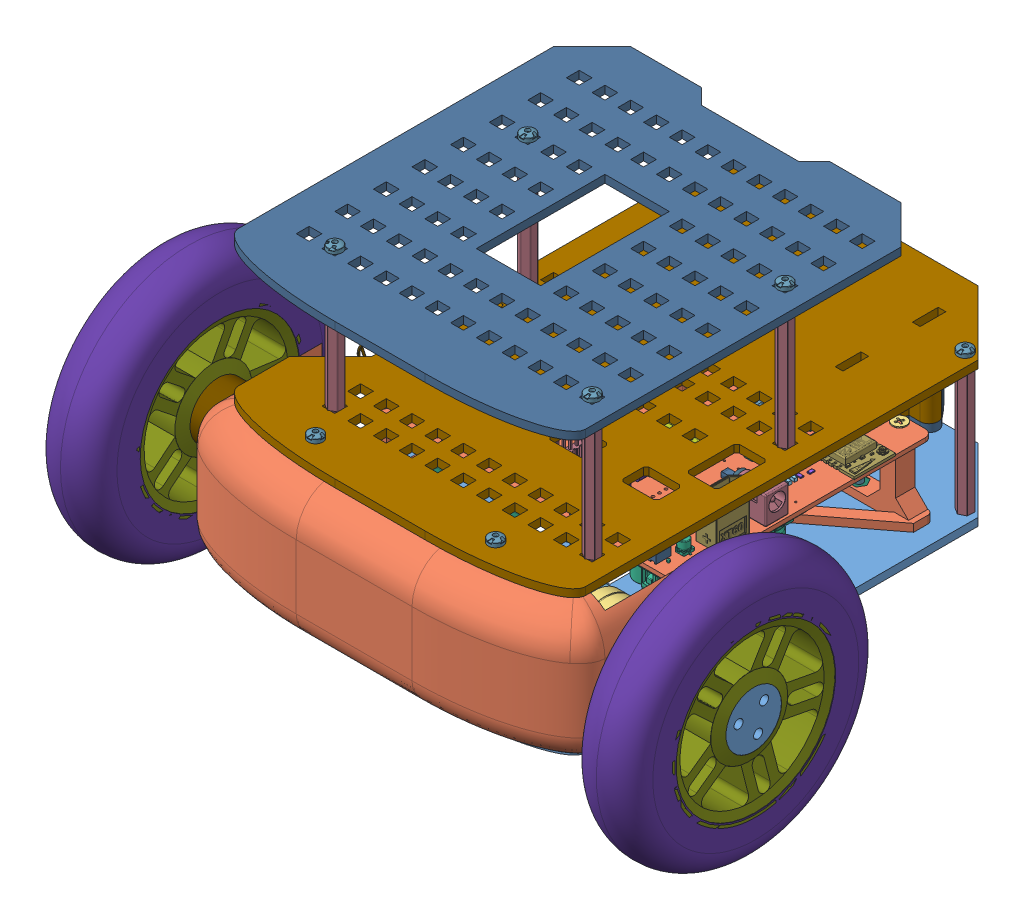
SolidWorks assembly assembly_base, configuration Default. Lengths in mm.
Overall size (232.39 156.66 252.89).
353 component instances, 65 part files, 83 mates.
Components (placement in the parent):
- base_noah-1: base_noah [Predeterminado] at (74.3097 87.0427 151.4169) size (135.31 3.5 190.25)
- assembly_front-1: assembly_front [Default] at (17.489 26.6548 114.6215) size (173 50.11 66.16)
  - front_noah-1: front_noah [Predeterminado] at (56.8207 63.3879 111.7954) size (155.37 50.11 66.16)
  - JA25-371-12V-1: JA25-371-12V [Predeterminado] at (89.756 81.55 118.7577) x (0 0 -1) z (1 0 0) size (25 25 76.39)
    - Gearbox-1: Gearbox [Predeterminado] at (16.9623 5.2379 20.5646) size (25 25 21)
    - hub-1: hub [Predeterminado] at (16.9623 5.2379 39.5646) x (0.985611 -0.169031 0) z (0 0 1) size (6.95 6.95 4.5)
    - Motor-1: Motor [Predeterminado] at (16.9623 5.2379 -9.9354) size (24.2 24.2 30.5)
    - Axis-1: Axis [Predeterminado] at (16.9623 5.2379 39.5646) x (0.853161 0.521648 0) z (0 0 1) size (4 4 14)
    - PCB-1: PCB [Predeterminado] at (16.9623 5.2379 -11.4354) x (-1 0 0) z (0 0 -1) size (23 23 4.73)
    - Magnet-1: Magnet [Predeterminado] at (16.9623 5.2379 -17.3254) x (-0.17817 -0.984 0) z (0 0 -1) size (14.2 14.2 15.5)
  - JA25-371-12V-2: JA25-371-12V [Predeterminado] at (23.8853 81.55 84.8331) x (0 0 1) z (-1 0 0) size (25 25 76.39)
    - Gearbox-1: Gearbox [Predeterminado] at (16.9623 5.2379 20.5646) size (25 25 21)
    - hub-1: hub [Predeterminado] at (16.9623 5.2379 39.5646) x (0.985611 -0.169031 0) z (0 0 1) size (6.95 6.95 4.5)
    - Motor-1: Motor [Predeterminado] at (16.9623 5.2379 -9.9354) size (24.2 24.2 30.5)
    - Axis-1: Axis [Predeterminado] at (16.9623 5.2379 39.5646) x (0.853161 0.521648 0) z (0 0 1) size (4 4 14)
    - PCB-1: PCB [Predeterminado] at (16.9623 5.2379 -11.4354) x (-1 0 0) z (0 0 -1) size (23 23 4.73)
    - Magnet-1: Magnet [Predeterminado] at (16.9623 5.2379 -17.3254) x (-0.17817 -0.984 0) z (0 0 -1) size (14.2 14.2 15.5)
  - pan head cross collar screw_din-1: pan head cross collar screw_din [DIN 967 - M3 x 10 - Z --- 9C] at (-23.0293 86.7879 93.0454) size (12.25 7.5 7.5) (hidden)
  - pan head cross collar screw_din-2: pan head cross collar screw_din [DIN 967 - M3 x 10 - Z --- 9C] at (-23.0293 86.7879 110.5454) size (12.25 7.5 7.5) (hidden)
  - pan head cross collar screw_din-3: pan head cross collar screw_din [DIN 967 - M3 x 10 - Z --- 9C] at (136.6707 86.7879 93.0454) x (-1 0 0) z (0 -0.670219 0.742163) size (12.25 7.5 7.5) (hidden)
  - pan head cross collar screw_din-4: pan head cross collar screw_din [DIN 967 - M3 x 10 - Z --- 9C] at (136.6707 86.7879 110.5454) x (-1 0 0) z (0 -0.948777 -0.315948) size (12.25 7.5 7.5) (hidden)
- CasterJoint-1: CasterJoint [Default] at (94.6449 133.9119 11.2642) x (-1 0 0) z (0 0 1) size (61 48.46 48.78)
  - C000-1: C000 [Default] at (20.3352 23.8692 48.4027) size (61 17 46)
  - C001-1: C001 [Default] at (20.3352 23.8692 48.4027) size (61 16.32 46)
  - BALL6MM-1: BALL6MM [Predeterminado] at (22.8352 26.8692 52.7329) size (6 6 6)
  - BALL40MM-1: BALL40MM [Default] at (20.3352 49.3191 48.4027) x (0.992761 -0.035378 0.11478) z (-0.109645 0.123176 0.986309) size (40 40 40)
  - BALL6MM-2: BALL6MM [Predeterminado] at (22.8352 26.8692 44.0726) size (6 6 6)
  - BALL6MM-3: BALL6MM [Predeterminado] at (15.3352 26.8692 48.4027) size (6 6 6)
  - pan head cross collar screw_din-1: pan head cross collar screw_din [DIN 967 - M3 x 10 - Z --- 9C] at (-6.6648 46.2192 48.6527) x (0 -1 0) z (0.01313 0 0.999914) size (12.25 7.5 7.5) (hidden)
  - pan head cross collar screw_din-2: pan head cross collar screw_din [DIN 967 - M3 x 10 - Z --- 9C] at (47.3352 46.2192 48.6527) x (0 -1 0) z (0 0 1) size (12.25 7.5 7.5) (hidden)
- Spacer50mm-1: Spacer50mm [Varsayılan] at (136.8097 140.0427 81.4169) x (-0.837169 0 -0.546944) z (-0.546944 0 0.837169) size (5.71 56.2 5)
- Spacer50mm-3: Spacer50mm [Varsayılan] at (27.8097 140.0427 68.4169) x (-0.837169 0 -0.546944) z (-0.546944 0 0.837169) size (5.71 56.2 5)
- pan head cross recess screw_din-1: pan head cross recess screw_din [DIN EN ISO 7045 - M3 x 10 - Z - 10N] at (124.3097 84.6427 236.4169) x (0 1 0) z (0 0 1) size (12.31 5.6 5.6)
- pan head cross recess screw_din-2: pan head cross recess screw_din [DIN EN ISO 7045 - M3 x 10 - Z - 10N] at (24.3097 84.6427 236.4169) x (0 1 0) z (0.855611 0 0.517619) size (12.31 5.6 5.6)
- pan head cross recess screw_din-3: pan head cross recess screw_din [DIN EN ISO 7045 - M3 x 10 - Z - 10N] at (101.3097 84.6427 59.9169) x (0 1 0) z (0 0 1) size (12.31 5.6 5.6)
- pan head cross recess screw_din-4: pan head cross recess screw_din [DIN EN ISO 7045 - M3 x 10 - Z - 10N] at (101.8097 84.6427 201.4169) x (0 1 0) z (0 0 1) size (12.31 5.6 5.6)
- pan head cross recess screw_din-5: pan head cross recess screw_din [DIN EN ISO 7045 - M3 x 10 - Z - 10N] at (46.8097 84.6427 201.4169) x (0 1 0) z (0 0 1) size (12.31 5.6 5.6)
- pan head cross recess screw_din-6: pan head cross recess screw_din [DIN EN ISO 7045 - M3 x 10 - Z - 10N] at (47.3097 84.6427 59.9169) x (0 1 0) z (0.112447 0 0.993658) size (12.31 5.6 5.6)
- hex thin nut gradeb_din-1: hex thin nut gradeb_din [Hexagon Nut ISO 4036 - M3 - C] at (27.8097 85.2427 68.4169) x (1 0 0) z (0 -1 0) size (5.5 6.35 1.8)
- hex thin nut gradeb_din-2: hex thin nut gradeb_din [Hexagon Nut ISO 4036 - M3 - C] at (136.8097 85.2427 81.4169) x (1 0 0) z (0 -1 0) size (5.5 6.35 1.8)
- TuxsWheel100mm-1: TuxsWheel100mm [Default] at (255.3766 117.299 278.9192) x (0 0.731903 -0.681409) z (-1 0 0) size (114.18 114.18 36.69)
  - B02-1: B02 [Default] at (39.7671 48.3733 64.9228) size (90.04 90.04 24)
  - B021-1: B021 [Default] at (39.7671 48.3733 64.9228) x (0.988174 0.153337 0) z (0 0 1) size (100.02 100.02 24.11)
  - Adapter1-1: Adapter1 [Default] at (39.7671 48.3733 72.3069) x (0 -1 0) z (0 0 1) size (21.7 21.7 29.26)
  - Adapter2-1: Adapter2 [Default] at (39.7671 48.3733 65.8069) x (0 -1 0) z (0 0 1) size (21.7 21.7 6.5)
  - countersunk flat head cross recess screw_din-6: countersunk flat head cross recess screw_din [DIN EN ISO 7046-1 - M3 x 10 - Z - 10C] at (51.0178 48.3733 97.0669) x (-1 0 0) z (0 -0.928088 -0.37236) size (10 5.5 5.5) (hidden)
  - countersunk flat head cross recess screw_din-7: countersunk flat head cross recess screw_din [DIN EN ISO 7046-1 - M3 x 10 - Z - 10C] at (28.4595 48.3733 97.0669) x (1 0 0) z (0 0.306192 0.95197) size (10 5.5 5.5) (hidden)
  - countersunk flat head cross recess screw_din-8: countersunk flat head cross recess screw_din [DIN EN ISO 7046-1 - M3 x 10 - Z - 10C] at (36.7671 53.5694 65.4069) x (0 0 1) z (-0.331366 0.943502 0) size (10 5.5 5.5) (hidden)
  - countersunk flat head cross recess screw_din-9: countersunk flat head cross recess screw_din [DIN EN ISO 7046-1 - M3 x 10 - Z - 10C] at (36.7671 43.1771 65.4069) x (0 0 1) z (-0.394756 0.918786 0) size (10 5.5 5.5) (hidden)
  - countersunk flat head cross recess screw_din-10: countersunk flat head cross recess screw_din [DIN EN ISO 7046-1 - M3 x 10 - Z - 10C] at (45.7671 48.3733 65.4069) x (0 0 1) z (0.637808 -0.770196 0) size (10 5.5 5.5) (hidden)
  - hex thin nut gradeb_din-1: hex thin nut gradeb_din [Hexagon Nut ISO 4036 - M3 - C] at (33.3451 48.3733 97.0669) x (0 -1 0) z (-1 0 0) size (5.5 6.35 1.8) (hidden)
  - hex thin nut gradeb_din-2: hex thin nut gradeb_din [Hexagon Nut ISO 4036 - M3 - C] at (44.1892 48.3733 97.0669) x (0 -1 0) z (-1 0 0) size (5.5 6.35 1.8) (hidden)
- TuxsWheel100mm-2: TuxsWheel100mm [Default] at (-106.7572 70.8598 170.5029) x (0 0.998218 -0.059675) z (1 0 0) size (114.18 114.18 36.69)
  - B02-1: B02 [Default] at (39.7671 48.3733 64.9228) size (90.04 90.04 24)
  - B021-1: B021 [Default] at (39.7671 48.3733 64.9228) x (0.988174 0.153337 0) z (0 0 1) size (100.02 100.02 24.11)
  - Adapter1-1: Adapter1 [Default] at (39.7671 48.3733 72.3069) x (0 -1 0) z (0 0 1) size (21.7 21.7 29.26)
  - Adapter2-1: Adapter2 [Default] at (39.7671 48.3733 65.8069) x (0 -1 0) z (0 0 1) size (21.7 21.7 6.5)
  - countersunk flat head cross recess screw_din-6: countersunk flat head cross recess screw_din [DIN EN ISO 7046-1 - M3 x 10 - Z - 10C] at (51.0178 48.3733 97.0669) x (-1 0 0) z (0 -0.928088 -0.37236) size (10 5.5 5.5) (hidden)
  - countersunk flat head cross recess screw_din-7: countersunk flat head cross recess screw_din [DIN EN ISO 7046-1 - M3 x 10 - Z - 10C] at (28.4595 48.3733 97.0669) x (1 0 0) z (0 0.306192 0.95197) size (10 5.5 5.5) (hidden)
  - countersunk flat head cross recess screw_din-8: countersunk flat head cross recess screw_din [DIN EN ISO 7046-1 - M3 x 10 - Z - 10C] at (36.7671 53.5694 65.4069) x (0 0 1) z (-0.331366 0.943502 0) size (10 5.5 5.5) (hidden)
  - countersunk flat head cross recess screw_din-9: countersunk flat head cross recess screw_din [DIN EN ISO 7046-1 - M3 x 10 - Z - 10C] at (36.7671 43.1771 65.4069) x (0 0 1) z (-0.394756 0.918786 0) size (10 5.5 5.5) (hidden)
  - countersunk flat head cross recess screw_din-10: countersunk flat head cross recess screw_din [DIN EN ISO 7046-1 - M3 x 10 - Z - 10C] at (45.7671 48.3733 65.4069) x (0 0 1) z (0.637808 -0.770196 0) size (10 5.5 5.5) (hidden)
  - hex thin nut gradeb_din-1: hex thin nut gradeb_din [Hexagon Nut ISO 4036 - M3 - C] at (33.3451 48.3733 97.0669) x (0 -1 0) z (-1 0 0) size (5.5 6.35 1.8) (hidden)
  - hex thin nut gradeb_din-2: hex thin nut gradeb_din [Hexagon Nut ISO 4036 - M3 - C] at (44.1892 48.3733 97.0669) x (0 -1 0) z (-1 0 0) size (5.5 6.35 1.8) (hidden)
- assembly_pcb_support-1: assembly_pcb_support [Default] at (108.2926 25.3704 228.3275) x (-1 0 0) z (0 0 -1) size (150.42 179.59 182.4)
  - pcb_holder_noah-1: pcb_holder_noah [Default] at (46.4357 64.6723 64.4341) size (120 28 100)
  - noah_v02-1: noah_v02 [Default] at (-116.0171 92.6723 -13.0895) x (1 0 0) z (0 1 0) size (125.96 104.91 49.76)
    - noah_v02.step-1: noah_v02.step [Default] at origin size (125.96 104.91 49.76)
      - IDC-Header_2x05_P2.54mm_Vertical.step-1: IDC-Header_2x05_P2.54mm_Vertical.step [Default] at (176.6 -132.6 1.65) x (-0.707107 0.707107 0) z (0 0 1) size (9.1 20.36 12.1)
        - SOLID.step-1: SOLID.step [Default] at origin size (9.1 20.36 12.1)
      - DFN-8-1EP_3x3mm_P0.5mm_EP1.66x2.38mm.step-1: DFN-8-1EP_3x3mm_P0.5mm_EP1.66x2.38mm.step [Default] at (105.305 -107.385 1.65) x (0 1 0) z (0 0 1) size (3 2.98 0.77)
        - SOLID-0.step-1: SOLID-0.step [Default] at origin size (3 2.98 0.77)
      - C_0805_2012Metric.step-1: C_0805_2012Metric.step [Default] at (160.4 -70.1 1.65) x (0 -1 0) z (0 0 1) size (2 1.25 1.25)
        - SOLID-1.step-1: SOLID-1.step [Default] at origin size (2 1.25 1.25)
      - CP_Elec_4x4.5.step-1: CP_Elec_4x4.5.step [Default] at (140.6 -65.3 1.65) x (0 -1 0) z (0 0 1) size (5.74 5.46 4.5)
        - SOLID-2.step-1: SOLID-2.step [Default] at origin size (5.74 5.46 4.5)
      - C_0805_2012Metric.step-2: C_0805_2012Metric.step [Default] at (115.6 -134.6 1.65) size (2 1.25 1.25)
        - SOLID-1.step-1: SOLID-1.step [Default] at origin size (2 1.25 1.25)
      - CP_Elec_4x4.5.step-2: CP_Elec_4x4.5.step [Default] at (114.6 -129.4 1.65) x (0 1 0) z (0 0 1) size (5.74 5.46 4.5)
        - SOLID-2.step-1: SOLID-2.step [Default] at origin size (5.74 5.46 4.5)
      - PinSocket_1x06_P2.54mm_Vertical.step-1: PinSocket_1x06_P2.54mm_Vertical.step [Default] at (153.2 -146.2 1.65) x (0 -1 0) z (0 0 1) size (2.54 15.24 10.1)
        - SOLID-3.step-1: SOLID-3.step [Default] at origin size (2.54 15.24 10.1)
      - PinSocket_2x06_P2.54mm_Vertical.step-1: PinSocket_2x06_P2.54mm_Vertical.step [Default] at (153.2 -142.6 1.65) x (0 -1 0) z (0 0 1) size (5.08 15.24 10.1)
        - SOLID-4.step-1: SOLID-4.step [Default] at origin size (5.08 15.24 10.1)
      - ublox_NEO-6M.step-1: ublox_NEO-6M.step [Default] at (181.8 -59.6 11.65) x (0 1 0) z (1 0 0) size (39.06 22.61 48.01)
        - COMPOUND.step-1: COMPOUND.step [Default] at origin size (39.06 22.61 48.01)
      - D_SMA.step-1: D_SMA.step [Default] at (198.4 -143.2 1.65) x (-1 0 0) z (0 0 1) size (5 2.7 2.22)
        - SOLID-5.step-1: SOLID-5.step [Default] at origin size (5 2.7 2.22)
      - PinHeader_1x03_P2.54mm_Vertical.step-1: PinHeader_1x03_P2.54mm_Vertical.step [Default] at (105.6 -147.4 1.65) x (-1 0 0) z (0 0 1) size (2.54 7.62 11.54)
        - SOLID-6.step-1: SOLID-6.step [Default] at origin size (2.54 7.62 11.54)
      - C_0805_2012Metric.step-3: C_0805_2012Metric.step [Default] at (101.3 -107.1 1.65) x (-1 0 0) z (0 0 1) size (2 1.25 1.25)
        - SOLID-1.step-1: SOLID-1.step [Default] at origin size (2 1.25 1.25)
      - C_0805_2012Metric.step-4: C_0805_2012Metric.step [Default] at (101.3 -104.8 1.65) x (-1 0 0) z (0 0 1) size (2 1.25 1.25)
        - SOLID-1.step-1: SOLID-1.step [Default] at origin size (2 1.25 1.25)
      - ESP07.step-1: ESP07.step [Default] at (101.6 -127.3 1.65) x (0 1 0) z (1 0 0) size (19.34 14.61 27.24)
        - COMPOUND-7.step-1: COMPOUND-7.step [Default] at origin size (19.34 14.61 27.24)
      - Power_Barrel_Connector_Jack_694106301002.step-1: Power_Barrel_Connector_Jack_694106301002.step [Default] at (104.13 -90.01 1.65) x (0 -1 0) z (0 0 1) size (9.49 14.48 14.52)
        - COMPOUND-8.step-1: COMPOUND-8.step [Default] at origin size (9.49 14.48 14.52)
      - GY-91.step-1: GY-91.step [Default] at (119 -134.7 9.65) size (14.4 21 11.75)
        - COMPOUND-9.step-1: COMPOUND-9.step [Default] at origin size (14.4 21 11.75)
      - Tact_Switch_4.5mm_SMT.step-1: Tact_Switch_4.5mm_SMT.step [Default] at (139.14 -127.61 1.65) x (0 1 0) z (0 0 1) size (7.5 4.5 4.2)
        - COMPOUND-10.step-1: COMPOUND-10.step [Default] at origin size (7.5 4.5 4.2)
      - Tact_Switch_4.5mm_SMT.step-2: Tact_Switch_4.5mm_SMT.step [Default] at (167.3 -90.93 1.65) x (0 -1 0) z (0 0 1) size (7.5 4.5 4.2)
        - COMPOUND-10.step-1: COMPOUND-10.step [Default] at origin size (7.5 4.5 4.2)
      - tb5p-2p_p5_l10_w7-6_h10.step-1: tb5p-2p_p5_l10_w7-6_h10.step [Default] at (205.55 -62.68 6.65) x (0 1 0) z (1 0 0) size (10.6 14.1 7.6)
        - COMPOUND-11.step-1: COMPOUND-11.step [Default] at origin size (10.6 14.1 7.6)
      - SW_DIP_SPSTx02_Slide_6.7x6.64mm_W7.62mm_P2.54mm_LowProfile.step-1: SW_DIP_SPSTx02_Slide_6.7x6.64mm_W7.62mm_P2.54mm_LowProfile.step [Default] at (131.45 -139.55 1.65) x (-1 0 0) z (0 0 1) size (6.64 7.82 6)
        - SOLID-12.step-1: SOLID-12.step [Default] at origin size (6.64 7.82 6)
      - LQFP-100_14x14mm_P0.5mm.step-1: LQFP-100_14x14mm_P0.5mm.step [Default] at (161.4 -120.1 1.65) x (0.707107 -0.707107 0) z (0 0 1) size (16 16 1.5)
        - SOLID-13.step-1: SOLID-13.step [Default] at origin size (16 16 1.5)
      - USB_Mini-B_Lumberg_2486_01_Horizontal.step-1: USB_Mini-B_Lumberg_2486_01_Horizontal.step [Default] at (203.6 -123.9 1.65) x (0 1 0) z (0 0 1) size (9.9 9.21 5)
        - SOLID-14.step-1: SOLID-14.step [Default] at origin size (9.9 9.21 5)
      - Crystal_HC49-U_Vertical.step-1: Crystal_HC49-U_Vertical.step [Default] at (151.7 -106.6 1.65) x (-0.707107 -0.707107 0) z (0 0 1) size (10.9 4.65 16)
        - SOLID-15.step-1: SOLID-15.step [Default] at origin size (10.9 4.65 16)
      - SOIC-8_3.9x4.9mm_P1.27mm.step-1: SOIC-8_3.9x4.9mm_P1.27mm.step [Default] at (190.4 -107.7 1.65) size (6 4.9 1.75)
        - SOLID-16.step-1: SOLID-16.step [Default] at origin size (6 4.9 1.75)
      - SOT-23-5.step-1: SOT-23-5.step [Default] at (201.6 -138 1.65) size (2.8 2.9 1.55)
        - SOLID-17.step-1: SOLID-17.step [Default] at origin size (2.8 2.9 1.55)
      - SOT-23-6.step-1: SOT-23-6.step [Default] at (193.5 -124.3 1.65) size (2.8 2.9 1.55)
        - SOLID-18.step-1: SOLID-18.step [Default] at origin size (2.8 2.9 1.55)
      - XL4015_StepDown_DC-DC_5A_(CC-CV)_v1.step-1: XL4015_StepDown_DC-DC_5A_(CC-CV)_v1.step [Default] at (119.3 -102.3 -0.05) x (0 1 0) z (0 0 -1) size (51 26 18.15)
        - COMPOUND-19.step-1: COMPOUND-19.step [Default] at origin size (51 26 18.15)
      - XL4015_StepDown_DC-DC_5A_(CC-CV)_v1.step-2: XL4015_StepDown_DC-DC_5A_(CC-CV)_v1.step [Default] at (147.1 -102.4 -0.05) x (0 1 0) z (0 0 -1) size (51 26 18.15)
        - COMPOUND-19.step-1: COMPOUND-19.step [Default] at origin size (51 26 18.15)
      - XL4015_StepDown_DC-DC_5A_(CC-CV)_v1.step-3: XL4015_StepDown_DC-DC_5A_(CC-CV)_v1.step [Default] at (174.9 -102.3 -0.05) x (0 1 0) z (0 0 -1) size (51 26 18.15)
        - COMPOUND-19.step-1: COMPOUND-19.step [Default] at origin size (51 26 18.15)
      - XL4015_StepDown_DC-DC_5A_(CC-CV)_v1.step-4: XL4015_StepDown_DC-DC_5A_(CC-CV)_v1.step [Default] at (91.5 -102.3 -0.05) x (0 1 0) z (0 0 -1) size (51 26 18.15)
        - COMPOUND-19.step-1: COMPOUND-19.step [Default] at origin size (51 26 18.15)
      - TB6612FNG_Motor_Driver.step-1: TB6612FNG_Motor_Driver.step [Default] at (130.68 -80.59 11.65) x (0 0 1) z (1 0 0) size (3.57 20.98 20.9)
        - SOLID-20.step-1: SOLID-20.step [Default] at origin size (3.57 20.98 20.9)
      - R_0805_2012Metric.step-1: R_0805_2012Metric.step [Default] at (168.4 -107.4 1.65) x (0.707107 -0.707107 0) z (0 0 1) size (2 1.2 0.45)
        - SOLID-21.step-1: SOLID-21.step [Default] at origin size (2 1.2 0.45)
      - R_0805_2012Metric.step-2: R_0805_2012Metric.step [Default] at (200.7 -105.4 1.65) x (0 1 0) z (0 0 1) size (2 1.2 0.45)
        - SOLID-21.step-1: SOLID-21.step [Default] at origin size (2 1.2 0.45)
      - R_0805_2012Metric.step-3: R_0805_2012Metric.step [Default] at (200.7 -109.4 1.65) x (0 -1 0) z (0 0 1) size (2 1.2 0.45)
        - SOLID-21.step-1: SOLID-21.step [Default] at origin size (2 1.2 0.45)
      - R_0805_2012Metric.step-4: R_0805_2012Metric.step [Default] at (197.3 -105.4 1.65) x (0 1 0) z (0 0 1) size (2 1.2 0.45)
        - SOLID-21.step-1: SOLID-21.step [Default] at origin size (2 1.2 0.45)
      - R_0805_2012Metric.step-5: R_0805_2012Metric.step [Default] at (197.3 -109.4 1.65) x (0 -1 0) z (0 0 1) size (2 1.2 0.45)
        - SOLID-21.step-1: SOLID-21.step [Default] at origin size (2 1.2 0.45)
      - R_0805_2012Metric.step-6: R_0805_2012Metric.step [Default] at (192.1 -103.5 1.65) size (2 1.2 0.45)
        - SOLID-21.step-1: SOLID-21.step [Default] at origin size (2 1.2 0.45)
      - R_0805_2012Metric.step-7: R_0805_2012Metric.step [Default] at (201.6 -131.9 1.65) x (-1 0 0) z (0 0 1) size (2 1.2 0.45)
        - SOLID-21.step-1: SOLID-21.step [Default] at origin size (2 1.2 0.45)
      - R_0805_2012Metric.step-8: R_0805_2012Metric.step [Default] at (193.5 -120.9 1.65) size (2 1.2 0.45)
        - SOLID-21.step-1: SOLID-21.step [Default] at origin size (2 1.2 0.45)
      - R_0805_2012Metric.step-9: R_0805_2012Metric.step [Default] at (192.9 -127.5 1.65) x (-1 0 0) z (0 0 1) size (2 1.2 0.45)
        - SOLID-21.step-1: SOLID-21.step [Default] at origin size (2 1.2 0.45)
      - R_0805_2012Metric.step-10: R_0805_2012Metric.step [Default] at (192.9 -129.9 1.65) size (2 1.2 0.45)
        - SOLID-21.step-1: SOLID-21.step [Default] at origin size (2 1.2 0.45)
      - R_0805_2012Metric.step-11: R_0805_2012Metric.step [Default] at (110.6 -141.6 1.65) size (2 1.2 0.45)
        - SOLID-21.step-1: SOLID-21.step [Default] at origin size (2 1.2 0.45)
      - R_0805_2012Metric.step-12: R_0805_2012Metric.step [Default] at (177.2 -71.9 1.65) x (-1 0 0) z (0 0 1) size (2 1.2 0.45)
        - SOLID-21.step-1: SOLID-21.step [Default] at origin size (2 1.2 0.45)
      - R_0805_2012Metric.step-13: R_0805_2012Metric.step [Default] at (177.2 -65.3 1.65) x (-1 0 0) z (0 0 1) size (2 1.2 0.45)
        - SOLID-21.step-1: SOLID-21.step [Default] at origin size (2 1.2 0.45)
      - R_0805_2012Metric.step-14: R_0805_2012Metric.step [Default] at (177.2 -69.7 1.65) x (-1 0 0) z (0 0 1) size (2 1.2 0.45)
        - SOLID-21.step-1: SOLID-21.step [Default] at origin size (2 1.2 0.45)
      - R_0805_2012Metric.step-15: R_0805_2012Metric.step [Default] at (177.2 -67.5 1.65) x (-1 0 0) z (0 0 1) size (2 1.2 0.45)
        - SOLID-21.step-1: SOLID-21.step [Default] at origin size (2 1.2 0.45)
      - R_0805_2012Metric.step-16: R_0805_2012Metric.step [Default] at (165.3 -97.8 1.65) x (0 1 0) z (0 0 1) size (2 1.2 0.45)
        - SOLID-21.step-1: SOLID-21.step [Default] at origin size (2 1.2 0.45)
      - R_0805_2012Metric.step-17: R_0805_2012Metric.step [Default] at (152.4 -93.8 1.65) x (0 -1 0) z (0 0 1) size (2 1.2 0.45)
        - SOLID-21.step-1: SOLID-21.step [Default] at origin size (2 1.2 0.45)
      - R_0805_2012Metric.step-18: R_0805_2012Metric.step [Default] at (155.2 -93.8 1.65) x (0 -1 0) z (0 0 1) size (2 1.2 0.45)
        - SOLID-21.step-1: SOLID-21.step [Default] at origin size (2 1.2 0.45)
      - R_0805_2012Metric.step-19: R_0805_2012Metric.step [Default] at (192.9 -132.2 1.65) x (-1 0 0) z (0 0 1) size (2 1.2 0.45)
        - SOLID-21.step-1: SOLID-21.step [Default] at origin size (2 1.2 0.45)
      - R_0805_2012Metric.step-20: R_0805_2012Metric.step [Default] at (169 -104.8 1.65) x (0.707107 -0.707107 0) z (0 0 1) size (2 1.2 0.45)
        - SOLID-21.step-1: SOLID-21.step [Default] at origin size (2 1.2 0.45)
      - R_0805_2012Metric.step-21: R_0805_2012Metric.step [Default] at (174.7 -105.9 1.65) size (2 1.2 0.45)
        - SOLID-21.step-1: SOLID-21.step [Default] at origin size (2 1.2 0.45)
      - R_0805_2012Metric.step-22: R_0805_2012Metric.step [Default] at (111.4 -74.4 1.65) x (0 1 0) z (0 0 1) size (2 1.2 0.45)
        - SOLID-21.step-1: SOLID-21.step [Default] at origin size (2 1.2 0.45)
      - R_0805_2012Metric.step-23: R_0805_2012Metric.step [Default] at (110.4 -77.6 1.65) x (-1 0 0) z (0 0 1) size (2 1.2 0.45)
        - SOLID-21.step-1: SOLID-21.step [Default] at origin size (2 1.2 0.45)
      - R_0805_2012Metric.step-24: R_0805_2012Metric.step [Default] at (101.3 -109.5 1.65) size (2 1.2 0.45)
        - SOLID-21.step-1: SOLID-21.step [Default] at origin size (2 1.2 0.45)
      - R_0805_2012Metric.step-25: R_0805_2012Metric.step [Default] at (100.5 -113.1 1.65) x (0 -1 0) z (0 0 1) size (2 1.2 0.45)
        - SOLID-21.step-1: SOLID-21.step [Default] at origin size (2 1.2 0.45)
      - R_0805_2012Metric.step-26: R_0805_2012Metric.step [Default] at (115.4 -147.6 1.65) size (2 1.2 0.45)
        - SOLID-21.step-1: SOLID-21.step [Default] at origin size (2 1.2 0.45)
      - R_0805_2012Metric.step-27: R_0805_2012Metric.step [Default] at (115.4 -145.4 1.65) size (2 1.2 0.45)
        - SOLID-21.step-1: SOLID-21.step [Default] at origin size (2 1.2 0.45)
      - R_0805_2012Metric.step-28: R_0805_2012Metric.step [Default] at (115.4 -143.2 1.65) size (2 1.2 0.45)
        - SOLID-21.step-1: SOLID-21.step [Default] at origin size (2 1.2 0.45)
      - R_0805_2012Metric.step-29: R_0805_2012Metric.step [Default] at (115.4 -141 1.65) size (2 1.2 0.45)
        - SOLID-21.step-1: SOLID-21.step [Default] at origin size (2 1.2 0.45)
      - R_2512_6332Metric.step-1: R_2512_6332Metric.step [Default] at (105.2 -100.8 1.65) size (6.3 3.2 0.6)
        - SOLID-22.step-1: SOLID-22.step [Default] at origin size (6.3 3.2 0.6)
      - R_0805_2012Metric.step-30: R_0805_2012Metric.step [Default] at (104 -112.2 1.65) x (-1 0 0) z (0 0 1) size (2 1.2 0.45)
        - SOLID-21.step-1: SOLID-21.step [Default] at origin size (2 1.2 0.45)
      - R_0805_2012Metric.step-31: R_0805_2012Metric.step [Default] at (104 -114.4 1.65) x (-1 0 0) z (0 0 1) size (2 1.2 0.45)
        - SOLID-21.step-1: SOLID-21.step [Default] at origin size (2 1.2 0.45)
      - R_0805_2012Metric.step-32: R_0805_2012Metric.step [Default] at (118.1 -81.9 1.65) x (-1 0 0) z (0 0 1) size (2 1.2 0.45)
        - SOLID-21.step-1: SOLID-21.step [Default] at origin size (2 1.2 0.45)
      - Molex_KK-254_AE-6410-04A_1x04_P2.54mm_Vertical.step-1: Molex_KK-254_AE-6410-04A_1x04_P2.54mm_Vertical.step [Default] at (205.6 -95.2 1.65) x (0 -1 0) z (0 0 1) size (10.16 5.8 15.26)
        - SOLID-23.step-1: SOLID-23.step [Default] at origin size (10.16 5.8 15.26)
      - Molex_KK-254_AE-6410-06A_1x06_P2.54mm_Vertical.step-1: Molex_KK-254_AE-6410-06A_1x06_P2.54mm_Vertical.step [Default] at (192 -144.6 1.65) x (-1 0 0) z (0 0 1) size (15.24 5.8 15.26)
        - SOLID-24.step-1: SOLID-24.step [Default] at origin size (15.24 5.8 15.26)
      - Molex_KK-254_AE-6410-04A_1x04_P2.54mm_Vertical.step-2: Molex_KK-254_AE-6410-04A_1x04_P2.54mm_Vertical.step [Default] at (205.6 -70.8 1.65) x (0 -1 0) z (0 0 1) size (10.16 5.8 15.26)
        - SOLID-23.step-1: SOLID-23.step [Default] at origin size (10.16 5.8 15.26)
      - Molex_KK-254_AE-6410-04A_1x04_P2.54mm_Vertical.step-3: Molex_KK-254_AE-6410-04A_1x04_P2.54mm_Vertical.step [Default] at (205.6 -107.4 1.65) x (0 -1 0) z (0 0 1) size (10.16 5.8 15.26)
        - SOLID-23.step-1: SOLID-23.step [Default] at origin size (10.16 5.8 15.26)
      - Molex_KK-254_AE-6410-04A_1x04_P2.54mm_Vertical.step-4: Molex_KK-254_AE-6410-04A_1x04_P2.54mm_Vertical.step [Default] at (205.6 -83 1.65) x (0 -1 0) z (0 0 1) size (10.16 5.8 15.26)
        - SOLID-23.step-1: SOLID-23.step [Default] at origin size (10.16 5.8 15.26)
      - PinHeader_1x03_P2.54mm_Vertical.step-2: PinHeader_1x03_P2.54mm_Vertical.step [Default] at (163.25 -146.15 1.65) x (-1 0 0) z (0 0 1) size (2.54 7.62 11.54)
        - SOLID-6.step-1: SOLID-6.step [Default] at origin size (2.54 7.62 11.54)
      - PinHeader_1x03_P2.54mm_Vertical.step-3: PinHeader_1x03_P2.54mm_Vertical.step [Default] at (167.05 -146.15 1.65) x (-1 0 0) z (0 0 1) size (2.54 7.62 11.54)
        - SOLID-6.step-1: SOLID-6.step [Default] at origin size (2.54 7.62 11.54)
      - PinHeader_1x03_P2.54mm_Vertical.step-4: PinHeader_1x03_P2.54mm_Vertical.step [Default] at (170.85 -146.15 1.65) x (-1 0 0) z (0 0 1) size (2.54 7.62 11.54)
        - SOLID-6.step-1: SOLID-6.step [Default] at origin size (2.54 7.62 11.54)
      - PinHeader_1x03_P2.54mm_Vertical.step-5: PinHeader_1x03_P2.54mm_Vertical.step [Default] at (174.65 -146.15 1.65) x (-1 0 0) z (0 0 1) size (2.54 7.62 11.54)
        - SOLID-6.step-1: SOLID-6.step [Default] at origin size (2.54 7.62 11.54)
      - Molex_KK-254_AE-6410-04A_1x04_P2.54mm_Vertical.step-5: Molex_KK-254_AE-6410-04A_1x04_P2.54mm_Vertical.step [Default] at (108.5 -54.8 1.65) x (-1 0 0) z (0 0 1) size (10.16 5.8 15.26)
        - SOLID-23.step-1: SOLID-23.step [Default] at origin size (10.16 5.8 15.26)
      - Molex_KK-254_AE-6410-04A_1x04_P2.54mm_Vertical.step-6: Molex_KK-254_AE-6410-04A_1x04_P2.54mm_Vertical.step [Default] at (163.9 -55 1.65) x (-1 0 0) z (0 0 1) size (10.16 5.8 15.26)
        - SOLID-23.step-1: SOLID-23.step [Default] at origin size (10.16 5.8 15.26)
      - XT60_Male_Connector.step-1: XT60_Male_Connector.step [Default] at (95.7 -75.4 17.65) x (0 1 0) z (-1 0 0) size (15.93 20.03 8.13)
        - COMPOUND-25.step-1: COMPOUND-25.step [Default] at origin size (15.93 20.03 8.13)
      - Molex_KK-254_AE-6410-04A_1x04_P2.54mm_Vertical.step-7: Molex_KK-254_AE-6410-04A_1x04_P2.54mm_Vertical.step [Default] at (136.5 -54.8 1.65) x (-1 0 0) z (0 0 1) size (10.16 5.8 15.26)
        - SOLID-23.step-1: SOLID-23.step [Default] at origin size (10.16 5.8 15.26)
      - Molex_KK-254_AE-6410-04A_1x04_P2.54mm_Vertical.step-8: Molex_KK-254_AE-6410-04A_1x04_P2.54mm_Vertical.step [Default] at (191.5 -54.9 1.65) x (-1 0 0) z (0 0 1) size (10.16 5.8 15.26)
        - SOLID-23.step-1: SOLID-23.step [Default] at origin size (10.16 5.8 15.26)
      - PinHeader_1x06_P2.54mm_Vertical.step-1: PinHeader_1x06_P2.54mm_Vertical.step [Default] at (152.6 -76.7 1.65) x (-1 0 0) z (0 0 1) size (2.54 15.24 11.54)
        - SOLID-26.step-1: SOLID-26.step [Default] at origin size (2.54 15.24 11.54)
      - PinHeader_1x06_P2.54mm_Vertical.step-2: PinHeader_1x06_P2.54mm_Vertical.step [Default] at (145.8 -76.74 1.65) x (-1 0 0) z (0 0 1) size (2.54 15.24 11.54)
        - SOLID-26.step-1: SOLID-26.step [Default] at origin size (2.54 15.24 11.54)
      - C_Disc_D7.5mm_W2.5mm_P5.00mm.step-1: C_Disc_D7.5mm_W2.5mm_P5.00mm.step [Default] at (108 -95 1.65) x (0 1 0) z (0 0 1) size (7.5 2.5 9.6)
        - SOLID-27.step-1: SOLID-27.step [Default] at origin size (7.5 2.5 9.6)
      - LED_1206_3216Metric.step-1: LED_1206_3216Metric.step [Default] at (206.8 -131.9 1.65) x (-1 0 0) z (0 0 1) size (3.2 1.6 1.1)
        - SOLID-28.step-1: SOLID-28.step [Default] at origin size (3.2 1.6 1.1)
      - D_SMA.step-2: D_SMA.step [Default] at (197.2 -136 1.65) x (0 1 0) z (0 0 1) size (5 2.7 2.22)
        - SOLID-5.step-1: SOLID-5.step [Default] at origin size (5 2.7 2.22)
      - D_SOD-323.step-1: D_SOD-323.step [Default] at (119.9 -147.5 1.65) size (2.5 1.25 1.1)
        - SOLID-29.step-1: SOLID-29.step [Default] at origin size (2.5 1.25 1.1)
      - D_SMA.step-3: D_SMA.step [Default] at (113.8 -95 1.65) x (-1 0 0) z (0 0 1) size (5 2.7 2.22)
        - SOLID-5.step-1: SOLID-5.step [Default] at origin size (5 2.7 2.22)
      - D_SMA.step-4: D_SMA.step [Default] at (115.8 -75.4 1.65) x (0 1 0) z (0 0 1) size (5 2.7 2.22)
        - SOLID-5.step-1: SOLID-5.step [Default] at origin size (5 2.7 2.22)
      - D_SMA.step-5: D_SMA.step [Default] at (104 -79.9 1.65) x (0 1 0) z (0 0 1) size (5 2.7 2.22)
        - SOLID-5.step-1: SOLID-5.step [Default] at origin size (5 2.7 2.22)
      - LED_1206_3216Metric.step-2: LED_1206_3216Metric.step [Default] at (152.4 -89 1.65) x (0 -1 0) z (0 0 1) size (3.2 1.6 1.1)
        - SOLID-28.step-1: SOLID-28.step [Default] at origin size (3.2 1.6 1.1)
      - LED_1206_3216Metric.step-3: LED_1206_3216Metric.step [Default] at (155.2 -89 1.65) x (0 -1 0) z (0 0 1) size (3.2 1.6 1.1)
        - SOLID-28.step-1: SOLID-28.step [Default] at origin size (3.2 1.6 1.1)
      - LED_1206_3216Metric.step-4: LED_1206_3216Metric.step [Default] at (192.4 -134.7 1.65) size (3.2 1.6 1.1)
        - SOLID-28.step-1: SOLID-28.step [Default] at origin size (3.2 1.6 1.1)
      - D_SOD-323.step-2: D_SOD-323.step [Default] at (110.7 -145.4 1.65) size (2.5 1.25 1.1)
        - SOLID-29.step-1: SOLID-29.step [Default] at origin size (2.5 1.25 1.1)
      - D_SOD-323.step-3: D_SOD-323.step [Default] at (119.9 -143.2 1.65) size (2.5 1.25 1.1)
        - SOLID-29.step-1: SOLID-29.step [Default] at origin size (2.5 1.25 1.1)
      - D_DO-41_SOD81_P10.16mm_Horizontal.step-1: D_DO-41_SOD81_P10.16mm_Horizontal.step [Default] at (131 -83.2 1.65) x (0 1 0) z (0 0 1) size (10.96 2.72 5.71)
        - SOLID-30.step-1: SOLID-30.step [Default] at origin size (10.96 2.72 5.71)
      - D_DO-41_SOD81_P10.16mm_Horizontal.step-2: D_DO-41_SOD81_P10.16mm_Horizontal.step [Default] at (136.1 -67.3 1.65) x (-1 0 0) z (0 0 1) size (10.96 2.72 5.71)
        - SOLID-30.step-1: SOLID-30.step [Default] at origin size (10.96 2.72 5.71)
      - D_DO-41_SOD81_P10.16mm_Horizontal.step-3: D_DO-41_SOD81_P10.16mm_Horizontal.step [Default] at (136.1 -63.7 1.65) x (-1 0 0) z (0 0 1) size (10.96 2.72 5.71)
        - SOLID-30.step-1: SOLID-30.step [Default] at origin size (10.96 2.72 5.71)
      - C_0805_2012Metric.step-5: C_0805_2012Metric.step [Default] at (160.8 -135.8 1.65) x (-0.707107 -0.707107 0) z (0 0 1) size (2 1.25 1.25)
        - SOLID-1.step-1: SOLID-1.step [Default] at origin size (2 1.25 1.25)
      - C_0603_1608Metric.step-1: C_0603_1608Metric.step [Default] at (193.96 -113.92 1.65) x (-1 0 0) z (0 0 1) size (1.6 0.8 0.8)
        - SOLID-31.step-1: SOLID-31.step [Default] at origin size (1.6 0.8 0.8)
      - C_0603_1608Metric.step-2: C_0603_1608Metric.step [Default] at (194 -112.2 1.65) x (-1 0 0) z (0 0 1) size (1.6 0.8 0.8)
        - SOLID-31.step-1: SOLID-31.step [Default] at origin size (1.6 0.8 0.8)
      - C_1206_3216Metric.step-1: C_1206_3216Metric.step [Default] at (206.8 -137.1 1.65) size (3.2 1.6 1.6)
        - SOLID-32.step-1: SOLID-32.step [Default] at origin size (3.2 1.6 1.6)
      - C_1206_3216Metric.step-2: C_1206_3216Metric.step [Default] at (206.8 -141.1 1.65) size (3.2 1.6 1.6)
        - SOLID-32.step-1: SOLID-32.step [Default] at origin size (3.2 1.6 1.6)
      - CP_Elec_4x4.5.step-3: CP_Elec_4x4.5.step [Default] at (116.6 -107.2 1.65) size (5.74 5.46 4.5)
        - SOLID-2.step-1: SOLID-2.step [Default] at origin size (5.74 5.46 4.5)
      - CP_Elec_4x4.5.step-4: CP_Elec_4x4.5.step [Default] at (98.8 -62 1.65) x (-1 0 0) z (0 0 1) size (5.74 5.46 4.5)
        - SOLID-2.step-1: SOLID-2.step [Default] at origin size (5.74 5.46 4.5)
      - C_0805_2012Metric.step-6: C_0805_2012Metric.step [Default] at (110.3 -84.1 1.65) size (2 1.25 1.25)
        - SOLID-1.step-1: SOLID-1.step [Default] at origin size (2 1.25 1.25)
      - CP_Elec_4x4.5.step-5: CP_Elec_4x4.5.step [Default] at (117.6 -60.5 1.65) x (-1 0 0) z (0 0 1) size (5.74 5.46 4.5)
        - SOLID-2.step-1: SOLID-2.step [Default] at origin size (5.74 5.46 4.5)
      - C_0805_2012Metric.step-7: C_0805_2012Metric.step [Default] at (168.1 -97.8 1.65) x (0 1 0) z (0 0 1) size (2 1.25 1.25)
        - SOLID-1.step-1: SOLID-1.step [Default] at origin size (2 1.25 1.25)
      - C_1206_3216Metric.step-3: C_1206_3216Metric.step [Default] at (176.8 -118 1.65) x (0.707107 0.707107 0) z (0 0 1) size (3.2 1.6 1.6)
        - SOLID-32.step-1: SOLID-32.step [Default] at origin size (3.2 1.6 1.6)
      - C_1206_3216Metric.step-4: C_1206_3216Metric.step [Default] at (178.6 -119.9 1.65) x (0.707107 0.707107 0) z (0 0 1) size (3.2 1.6 1.6)
        - SOLID-32.step-1: SOLID-32.step [Default] at origin size (3.2 1.6 1.6)
      - C_1206_3216Metric.step-5: C_1206_3216Metric.step [Default] at (157.3 -133.1 1.65) x (-0.707107 -0.707107 0) z (0 0 1) size (3.2 1.6 1.6)
        - SOLID-32.step-1: SOLID-32.step [Default] at origin size (3.2 1.6 1.6)
      - C_0603_1608Metric.step-3: C_0603_1608Metric.step [Default] at (145.2 -114.4 1.65) x (0.707107 -0.707107 0) z (0 0 1) size (1.6 0.8 0.8)
        - SOLID-31.step-1: SOLID-31.step [Default] at origin size (1.6 0.8 0.8)
      - C_0603_1608Metric.step-4: C_0603_1608Metric.step [Default] at (156.1 -103.5 1.65) x (0.707107 -0.707107 0) z (0 0 1) size (1.6 0.8 0.8)
